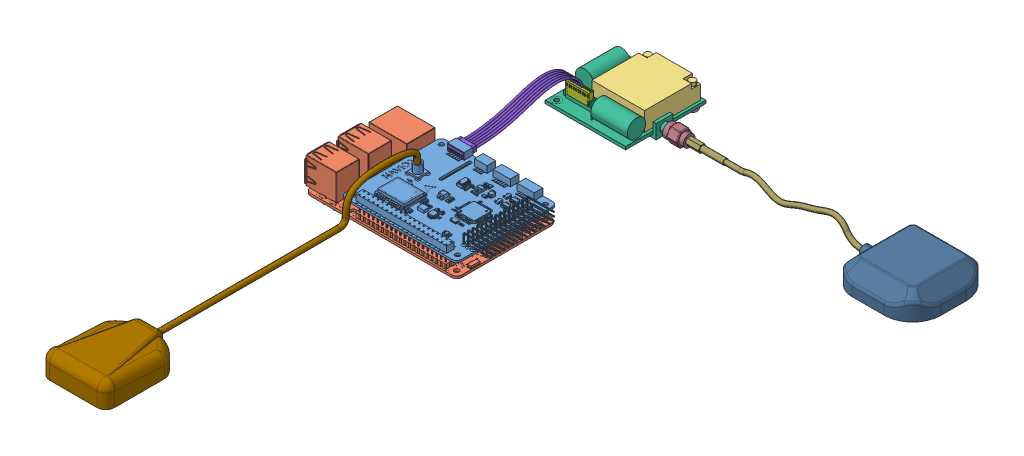
SolidWorks assembly ordinateur de bord, configuration Défaut. Lengths in mm.
Overall size (235.36 29.25 316.51).
18 component instances, 13 part files, 0 mates.
Components (placement in the parent):
- NAVIO2-1: NAVIO2 [Predeterminado] at (-2.1799 8.663 73.8182) size (73.82 8.2 56.43)
- raspberryPi3B-1: raspberryPi3B [Detailed] at (-12.2548 -0.3722 73.9221) x (-1 0 0) z (0 1 0) size (87.05 58.5 19.05)
- RockBLOCK_9603^ordinateur de bord-1: RockBLOCK_9603^ordinateur de bord [Défaut] at (-8.0137 -0.0406 -31.0806) x (0 0 -1) z (1 0 0) size (45.05 17 54.85) (virtual)
  - RockBLOCK V 3B^RockBLOCK_9603_ordinateur de bord-1: RockBLOCK V 3B^RockBLOCK_9603_ordinateur de bord [Défaut] at origin size (31.5 10.6 29.6) (virtual)
  - RockBLOCK V 3B-0^RockBLOCK_9603_ordinateur de bord-1: RockBLOCK V 3B-0^RockBLOCK_9603_ordinateur de bord [Défaut] at origin size (5.5 2.4 5.5) (virtual)
  - RockBLOCK V 3B-1^RockBLOCK_9603_ordinateur de bord-1: RockBLOCK V 3B-1^RockBLOCK_9603_ordinateur de bord [Défaut] at origin size (5.5 2.4 5.5) (virtual)
  - RockBLOCK V 3B-2^RockBLOCK_9603_ordinateur de bord-1: RockBLOCK V 3B-2^RockBLOCK_9603_ordinateur de bord [Défaut] at origin size (45.05 17 54.85) (virtual)
- HU-10^ordinateur de bord-2: HU-10^ordinateur de bord [Défaut] at (-30.9079 13.3327 -17.6067) x (1 0 0) z (0 -1 0) size (13.03 3.05 6.6) (virtual)
- HU-6^ordinateur de bord-1: HU-6^ordinateur de bord [Défaut] at (-15.3882 9.8124 53.38) x (-1 0 0) z (0 0 -1) size (8.9 11.37 67.92) (virtual)
- ANT-SH2^ordinateur de bord-1: ANT-SH2^ordinateur de bord [Défaut] at (-23.9216 -2.0661 240.4037) x (0 0 -1) z (1 0 0) size (194.46 25.81 36.51) (virtual)
- ANTENNA GPS^ordinateur de bord-1: ANTENNA GPS^ordinateur de bord [Défaut] at (155.5553 -4.9017 -28.6831) x (-1 0 0) z (0 1 0) size (159.5 46.02 14.84) (virtual)
  - RICEVITORE^ANTENNA GPS_ordinateur de bord-1: RICEVITORE^ANTENNA GPS_ordinateur de bord [Défaut] at origin size (50 46.02 14.25) (virtual)
  - GOMMINO ^ANTENNA GPS_ordinateur de bord-1: GOMMINO ^ANTENNA GPS_ordinateur de bord [Défaut] at origin size (2.57 2.57 1.6) (virtual)
  - GOMMINO ^ANTENNA GPS_ordinateur de bord-2: GOMMINO ^ANTENNA GPS_ordinateur de bord [Défaut] at (-32.5 -2.5 0) size (2.57 2.57 1.6) (virtual)
  - GOMMINO ^ANTENNA GPS_ordinateur de bord-3: GOMMINO ^ANTENNA GPS_ordinateur de bord [Défaut] at (0 -32.5 0) size (2.57 2.57 1.6) (virtual)
  - GOMMINO ^ANTENNA GPS_ordinateur de bord-4: GOMMINO ^ANTENNA GPS_ordinateur de bord [Défaut] at (-32.5 -30 0) size (2.57 2.57 1.6) (virtual)
  - FILO ^ANTENNA GPS_ordinateur de bord-1: FILO ^ANTENNA GPS_ordinateur de bord [Défaut] at (25 0 3) x (0 -1 0) z (0 0 1) size (4.33 107.45 12.65) (virtual)
  - JACK 3.5mm^ANTENNA GPS_ordinateur de bord-1: JACK 3.5mm^ANTENNA GPS_ordinateur de bord [Défaut] at (125.5 0 7) x (0 0 -1) z (1 0 0) size (8.01 9.08 11) (virtual)
